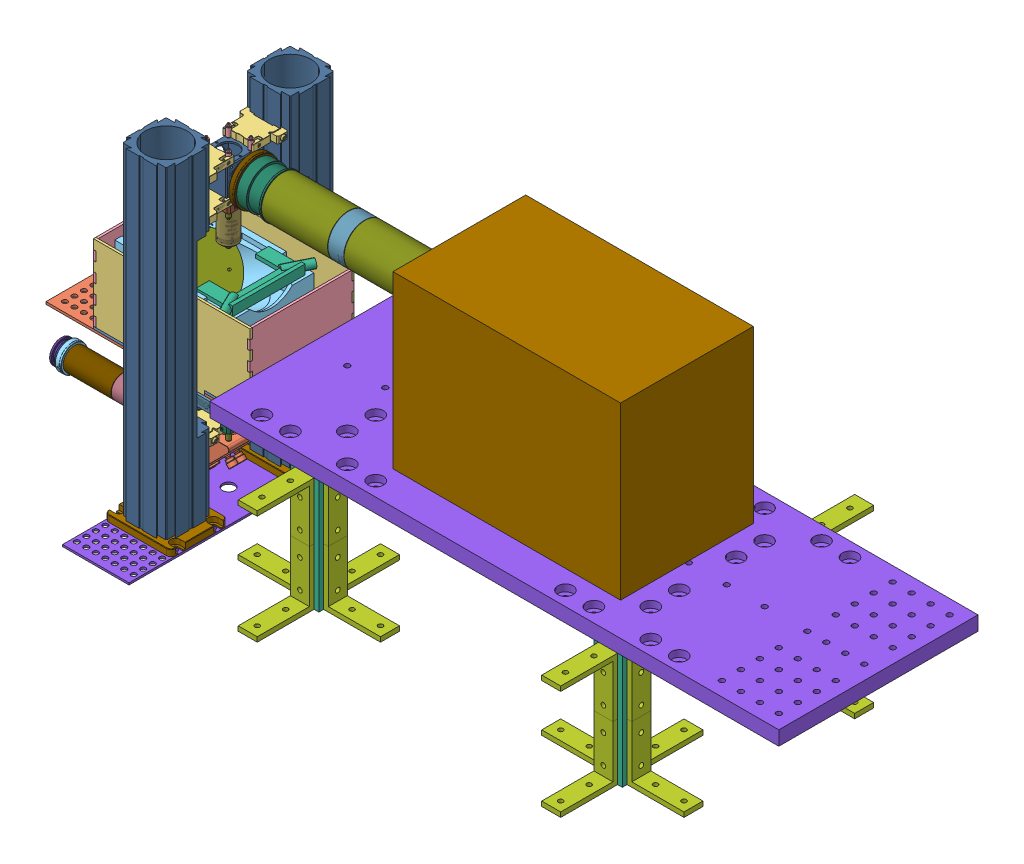
SolidWorks assembly Water Bath ABZ, configuration Default. Lengths in mm.
Overall size (1095.95 451.29 419.1).
114 component instances, 38 part files, 38 mates.
Components (placement in the parent):
- WB_0p125_BaseThreaded-1: WB_0p125_BaseThreaded [Default] at (0 3.175 0) size (209.55 3.17 139.7)
- WB_0p125_Base-1: WB_0p125_Base [Default] at origin size (273.05 3.17 139.7)
- WB_0p125_Long-1: WB_0p125_Long [Default] at (0 57.15 -69.85) size (209.55 107.95 3.17)
- WB_0p125_Long-2: WB_0p125_Long [Default] at (0 57.15 66.675) size (209.55 107.95 3.17)
- WB_0p125_Short-1: WB_0p125_Short [Default] at (101.6 57.15 0) x (0 0 1) z (0 1 0) size (139.7 3.17 107.95)
- WB_0p125_Short-2: WB_0p125_Short [Default] at (-104.775 57.15 0) x (0 0 1) z (0 1 0) size (139.7 3.17 107.95)
- 300 kHz Tank HP (5) Opticell-1: 300 kHz Tank HP (5) Opticell [Default] at (6.35 95.25 0) size (171.45 88.9 114.3)
- Opticell_Truncated-1: Opticell_Truncated [Default] at (23.9788 95.275 -0.195) size (53.01 12.75 129.72)
- HP Tx-1: HP Tx [Default] at (-41.775 64.925 0) x (0.498711 -0.863793 0.071763) z (-0.035882 0.062149 0.997422) size (83.8 58.17 83.8)
- Table SubAssembly-1: Table SubAssembly [Default] at (-31.75 -161.9485 0) x (0 0 -1) z (1 0 0) size (355.6 442.98 89.6)
  - Table-1: Table [Default] at origin size (355.6 2.54 88.9)
  - XT66P1-Solidworks-1: XT66P1-Solidworks [Default] at (-83.0224 2.286 37.592) x (-1 0 0) z (0 0 -1) size (76.2 8.89 89.28)
  - XT66P1-Solidworks-2: XT66P1-Solidworks [Default] at (83.0224 2.286 37.592) size (76.2 8.89 89.28)
  - KCB1-Solidworks-1: KCB1-Solidworks [Default] at (-24.13 99.7796 13.4747) x (0.000001 0 1) z (0 1 0) size (51.13 48.26 51.1) (hidden)
  - RCA1-Solidworks-1: RCA1-Solidworks [Default] at (-24.2926 205.6203 66.0649) x (0 0 -1) z (0 -1 0) size (56.5 73.55 8.89) (hidden)
  - RCA1-Solidworks-2: RCA1-Solidworks [Default] at (24.2926 108.2389 66.0649) x (0 0 -1) z (0 1 0) size (56.5 73.55 8.89) (hidden)
  - XT66-500-modified_v2-1: XT66-500-modified_v2 [Default] at (-83.0224 511.176 37.592) x (0 0 -1) z (0 -1 0) size (66.02 67.06 431.8)
  - XT66-500-modified_v2-2: XT66-500-modified_v2 [Default] at (83.0224 511.176 37.592) x (0 0 1) z (0 -1 0) size (66.02 67.06 431.8)
- Small Condenser Adjustable Sub-Assembly-1: Small Condenser Adjustable Sub-Assembly [Default] at (41.91 -37.4885 20.3199) x (0 -1 0) z (0 0 1) size (204.14 301.96 127)
  - LB1437-Solidworks-1: LB1437-Solidworks [Default] at (76.2 -223.413 -20.3199) x (0.879994 0 -0.474985) z (0 -1 0) size (25.4 25.4 3.05)
  - LB1761-Solidworks-1: LB1761-Solidworks [Default] at (76.2 -78.613 -20.3199) x (0.962182 0 -0.272406) z (0 -1 0) size (25.4 25.4 8.98)
  - SM1L40-Solidworks-1: SM1L40-Solidworks [Default] at (78.3398 -122.5422 -22.1696) x (-0.992854 0 -0.119336) z (0 1 0) size (30.48 30.48 105.41)
  - CSA1003-Solidworks-1: CSA1003-Solidworks [Default] at (47.6181 -122.449 -34.035) x (0 -1 0) z (0 0 1) size (71.12 13.97 71.12)
  - LCP02-Solidworks-1: LCP02-Solidworks [Default] at (20.32 -35.5599 -20.32) x (0 0 -1) z (1 0 0) size (70.75 70.61 12.7)
  - ER1-Solidworks-1: ER1-Solidworks [Default] at (36.8841 -51.9737 -4.6825) x (0 -0.925141 -0.379624) z (0 -0.379624 0.925141) size (5.99 30.48 5.99)
  - ER1-Solidworks-3: ER1-Solidworks [Default] at (36.8841 -50.6608 -33.7724) x (0 -0.769482 0.638668) z (0 0.638668 0.769482) size (5.99 30.48 5.99)
  - ER1-Solidworks-4: ER1-Solidworks [Default] at (41.8559 -21.5595 -36.5057) x (0 -0.998351 -0.057413) z (0 0.057413 -0.998351) size (5.99 30.48 5.99)
  - SM1T2-Solidworks-1: SM1T2-Solidworks [Default] at (76.2 -248.6152 -20.3199) x (0.998592 0 -0.053039) z (0 1 0) size (31.75 31.75 12.7)
  - SM1L25-Solidworks-1: SM1L25-Solidworks [Default] at (139.9124 -186.275 -15.6668) x (0 -1 0) z (-0.806632 0 -0.591053) size (67.31 30.48 30.48)
  - CP08-Solidworks-3: CP08-Solidworks [Default] at (76.2 -69.215 -20.3199) x (0 0 -1) z (0 1 0) size (41.5 40.64 8.89)
  - KCB1-Solidworks-2: KCB1-Solidworks [Default] at (100.33 -11.43 3.8101) x (-1 0 0) z (0 -1 0) size (51.13 48.26 51.1)
  - ER1-Solidworks-6: ER1-Solidworks [Default] at (36.8841 -20.7263 -3.7781) x (0 -0.795862 0.605478) z (0 0.605478 0.795862) size (5.99 30.48 5.99)
  - RCA2-Solidworks-1: RCA2-Solidworks [Default] at (68.2294 -49.0321 -29.2771) x (0 1 0) z (-1 0 0) size (56.73 41.06 8.89)
  - RCA2-Solidworks-2: RCA2-Solidworks [Default] at (68.2294 -22.0879 -11.3628) x (0 -1 0) z (-1 0 0) size (56.73 41.06 8.89)
  - ER05-Solidworks-1: ER05-Solidworks [Default] at (92.6015 -68.5259 -5.9839) x (0.310188 0 -0.950675) z (0.950675 0 0.310188) size (5.99 17.78 5.99)
  - ER05-Solidworks-2: ER05-Solidworks [Default] at (59.8613 -68.5259 -4.5371) x (-0.22668 0 0.973969) z (-0.973969 0 -0.22668) size (5.99 17.78 5.99)
  - ER05-Solidworks-3: ER05-Solidworks [Default] at (92.2659 -68.5259 -34.1935) size (5.99 17.78 5.99)
  - ER05-Solidworks-4: ER05-Solidworks [Default] at (59.7556 -68.5259 -34.7555) x (-0.375833 0 0.926687) z (-0.926687 0 -0.375833) size (5.99 17.78 5.99)
  - SM1D12D-Solidworks-1: SM1D12D-Solidworks [Default] at (81.3975 -244.783 -22.8892) x (0.973299 0 -0.22954) z (0 1 0) size (35.81 35.81 11.94)
  - SM1D12D-Solidworks-2: SM1D12D-Solidworks [Default] at (70.9424 -73.1298 -22.7639) x (-0.788375 0 -0.615195) z (0 1 0) size (35.81 35.81 11.94)
  - ER1-Solidworks-9: ER1-Solidworks [Default] at (15.1859 -4.2179 -49.5429) x (0 0.95877 -0.284182) z (0 0.284182 0.95877) size (5.99 30.48 5.99)
  - ER1-Solidworks-10: ER1-Solidworks [Default] at (15.1859 -64.6339 -49.076) x (0 0.993069 0.117534) z (0 -0.117534 0.993069) size (5.99 30.48 5.99)
  - ER1-Solidworks-11: ER1-Solidworks [Default] at (15.1859 -4.6008 10.8986) x (0 0.995869 0.090807) z (0 -0.090807 0.995869) size (5.99 30.48 5.99)
  - ER1-Solidworks-12: ER1-Solidworks [Default] at (15.1859 -64.2349 10.4858) x (0 0.96466 -0.263499) z (0 0.263499 0.96466) size (5.99 30.48 5.99)
  - OlympusCondenser-1: OlympusCondenser [Default] at (7.0104 -35.56 -20.3199) x (0 -1 0) z (0 0 -1) size (152.4 107.95 127) (hidden)
- Full Assembly Total Support-1: Full Assembly Total Support [Default] at (495.5495 41.6875 0) size (762 171.45 419.1)
  - Post SubAssembly-1: Post SubAssembly [Default] at (-254 -152.4 114.3) size (190.5 152.4 190.5)
    - Post-1: Post [Default] at origin size (38.1 152.4 38.1)
    - Hinge-1: Hinge [Default] at (-25.4 6.35 0) x (0 0 -1) z (0 -1 0) size (25.4 76.2 76.2)
    - Hinge-2: Hinge [Default] at (0 6.35 25.4) x (-1 0 0) z (0 -1 0) size (25.4 76.2 76.2)
    - Hinge-3: Hinge [Default] at (25.4 6.35 0) x (0 0 1) z (0 -1 0) size (25.4 76.2 76.2)
    - Hinge-4: Hinge [Default] at (0 6.35 -25.4) x (1 0 0) z (0 -1 0) size (25.4 76.2 76.2)
    - Hinge-5: Hinge [Default] at (25.4 146.05 0) x (0 0 1) z (-1 0 0) size (25.4 76.2 76.2)
    - Hinge-7: Hinge [Default] at (-25.4 146.05 0) x (0 0 -1) z (1 0 0) size (25.4 76.2 76.2)
    - Hinge-8: Hinge [Default] at (0 146.05 25.4) x (-1 0 0) z (0 0 -1) size (25.4 76.2 76.2)
    - Hinge-9: Hinge [Default] at (0 146.05 -25.4) size (25.4 76.2 76.2)
  - Post SubAssembly-2: Post SubAssembly [Default] at (-254 -152.4 -114.3) size (190.5 152.4 190.5)
    - Post-1: Post [Default] at origin size (38.1 152.4 38.1)
    - Hinge-1: Hinge [Default] at (-25.4 6.35 0) x (0 0 -1) z (0 -1 0) size (25.4 76.2 76.2)
    - Hinge-2: Hinge [Default] at (0 6.35 25.4) x (-1 0 0) z (0 -1 0) size (25.4 76.2 76.2)
    - Hinge-3: Hinge [Default] at (25.4 6.35 0) x (0 0 1) z (0 -1 0) size (25.4 76.2 76.2)
    - Hinge-4: Hinge [Default] at (0 6.35 -25.4) x (1 0 0) z (0 -1 0) size (25.4 76.2 76.2)
    - Hinge-5: Hinge [Default] at (25.4 146.05 0) x (0 0 1) z (-1 0 0) size (25.4 76.2 76.2)
    - Hinge-7: Hinge [Default] at (-25.4 146.05 0) x (0 0 -1) z (1 0 0) size (25.4 76.2 76.2)
    - Hinge-8: Hinge [Default] at (0 146.05 25.4) x (-1 0 0) z (0 0 -1) size (25.4 76.2 76.2)
    - Hinge-9: Hinge [Default] at (0 146.05 -25.4) size (25.4 76.2 76.2)
  - Post SubAssembly-3: Post SubAssembly [Default] at (152.4 -152.4 114.3) size (190.5 152.4 190.5)
    - Post-1: Post [Default] at origin size (38.1 152.4 38.1)
    - Hinge-1: Hinge [Default] at (-25.4 6.35 0) x (0 0 -1) z (0 -1 0) size (25.4 76.2 76.2)
    - Hinge-2: Hinge [Default] at (0 6.35 25.4) x (-1 0 0) z (0 -1 0) size (25.4 76.2 76.2)
    - Hinge-3: Hinge [Default] at (25.4 6.35 0) x (0 0 1) z (0 -1 0) size (25.4 76.2 76.2)
    - Hinge-4: Hinge [Default] at (0 6.35 -25.4) x (1 0 0) z (0 -1 0) size (25.4 76.2 76.2)
    - Hinge-5: Hinge [Default] at (25.4 146.05 0) x (0 0 1) z (-1 0 0) size (25.4 76.2 76.2)
    - Hinge-7: Hinge [Default] at (-25.4 146.05 0) x (0 0 -1) z (1 0 0) size (25.4 76.2 76.2)
    - Hinge-8: Hinge [Default] at (0 146.05 25.4) x (-1 0 0) z (0 0 -1) size (25.4 76.2 76.2)
    - Hinge-9: Hinge [Default] at (0 146.05 -25.4) size (25.4 76.2 76.2)
  - Post SubAssembly-4: Post SubAssembly [Default] at (152.4 -152.4 -114.3) size (190.5 152.4 190.5)
    - Post-1: Post [Default] at origin size (38.1 152.4 38.1)
    - Hinge-1: Hinge [Default] at (-25.4 6.35 0) x (0 0 -1) z (0 -1 0) size (25.4 76.2 76.2)
    - Hinge-2: Hinge [Default] at (0 6.35 25.4) x (-1 0 0) z (0 -1 0) size (25.4 76.2 76.2)
    - Hinge-3: Hinge [Default] at (25.4 6.35 0) x (0 0 1) z (0 -1 0) size (25.4 76.2 76.2)
    - Hinge-4: Hinge [Default] at (0 6.35 -25.4) x (1 0 0) z (0 -1 0) size (25.4 76.2 76.2)
    - Hinge-5: Hinge [Default] at (25.4 146.05 0) x (0 0 1) z (-1 0 0) size (25.4 76.2 76.2)
    - Hinge-7: Hinge [Default] at (-25.4 146.05 0) x (0 0 -1) z (1 0 0) size (25.4 76.2 76.2)
    - Hinge-8: Hinge [Default] at (0 146.05 25.4) x (-1 0 0) z (0 0 -1) size (25.4 76.2 76.2)
    - Hinge-9: Hinge [Default] at (0 146.05 -25.4) size (25.4 76.2 76.2)
  - Camera Shelf Full Support v2-1: Camera Shelf Full Support v2 [Default] at origin size (762 19.05 266.7)
- hpvx2-1: hpvx2 [Default] at (467.8011 60.7375 0.0468) size (311.15 228.6 177.8)
- Objective Sub-Assembly-1: Objective Sub-Assembly [Default] at (41.0423 -225.3982 114.3819) x (0 0 -1) z (0 -1 0) size (106.71 57.63 128.02)
  - CM1-DCH-Solidworks-1: CM1-DCH-Solidworks [Web Assembly] at (114.3818 -34.6924 -438.5894) x (0 -1 0) z (0 0 1) size (38.1 45.72 38.1)
  - CP16-Solidworks-1: CP16-Solidworks [Default] at (116.5677 -16.5858 -398.1348) x (0 -1 0) z (0 0 1) size (41.22 40.64 8.89)
  - RCA2-Solidworks-1: RCA2-Solidworks [Default] at (123.339 -21.2203 -499.1988) x (0 -1 0) z (0 0 1) size (56.73 41.06 8.89)
  - RCA2-Solidworks-2: RCA2-Solidworks [Default] at (105.4247 -48.1644 -499.1988) x (0 1 0) z (0 0 1) size (56.73 41.06 8.89)
  - N40X-NIR-Solidworks-1: N40X-NIR-Solidworks [Default] at (114.3819 -34.6923 -375.0894) x (0 0 1) z (0.875921 0.482454 0) size (61.98 27.94 27.94)
  - RCA2-Solidworks-3: RCA2-Solidworks [Default] at (105.4247 -48.1644 -452.2088) x (0 1 0) z (0 0 1) size (56.73 41.06 8.89)
  - RCA2-Solidworks-4: RCA2-Solidworks [Default] at (123.339 -21.2203 -452.2088) x (0 -1 0) z (0 0 1) size (56.73 41.06 8.89)
  - ER1-Solidworks-1: ER1-Solidworks [Default] at (100.293 -20.9473 -404.3535) x (-0.183947 -0.982936 0) z (0.982936 -0.183947 0) size (5.99 30.48 5.99)
  - ER1-Solidworks-2: ER1-Solidworks [Default] at (130.5299 -50.7349 -404.3535) x (0.020475 -0.99979 0) z (0.99979 0.020475 0) size (5.99 30.48 5.99)
  - ER1-Solidworks-3: ER1-Solidworks [Default] at (100.0093 -51.1105 -404.3535) x (-0.386185 -0.922421 0) z (0.922421 -0.386185 0) size (5.99 30.48 5.99)
  - ER1-Solidworks-4: ER1-Solidworks [Default] at (129.6817 -21.2139 -404.3535) x (-0.579753 -0.814792 0) z (0.814792 -0.579753 0) size (5.99 30.48 5.99)
  - ER05-Solidworks-1: ER05-Solidworks [Default] at (129.9725 -48.2584 -461.5035) x (0.933397 0.358845 0) z (-0.358845 0.933397 0) size (5.99 17.78 5.99)
  - ER05-Solidworks-2: ER05-Solidworks [Default] at (97.9162 -50.199 -461.5035) x (-0.886919 0.461926 0) z (-0.461926 -0.886919 0) size (5.99 17.78 5.99)
  - ER05-Solidworks-3: ER05-Solidworks [Default] at (128.9134 -21.1707 -461.5035) x (-0.900043 -0.4358 0) z (0.4358 -0.900043 0) size (5.99 17.78 5.99)
  - ER05-Solidworks-4: ER05-Solidworks [Default] at (100.2773 -18.4261 -461.5035) x (0.989892 0.141823 0) z (-0.141823 0.989892 0) size (5.99 17.78 5.99)
- Camera Sub-Assembly-1: Camera Sub-Assembly [Default] at (25.4 213.1913 0) x (0 -0.657803 -0.75319) z (-1 0 0) size (71.93 71.93 298.88)
  - SM2NFM2-Solidworks-1: SM2NFM2-Solidworks [Default] at (0 0 -285.6832) x (0 1 0) z (-1 0 0) size (63.5 16.37 63.5)
  - TTL200-S8-Solidworks-1: TTL200-S8-Solidworks [Default] at (0 0 -152.5317) size (55.88 55.88 28)
  - SM2V15-Solidworks-1: SM2V15-Solidworks [Default] at (18.0496 -29.8565 -288.422) x (0 0 -1) z (0.951776 0.306793 0) size (51.56 57.15 57.15)
  - SM2M35-Solidworks-1: SM2M35-Solidworks [Default] at (-10.7846 9.351 -219.5042) x (0.99081 -0.135264 0) z (0 0 1) size (55.88 55.88 88.9)
  - SM2M35-Solidworks-2: SM2M35-Solidworks [Default] at (-11.8362 7.9783 -108.9542) x (0.999895 -0.014459 0) z (0 0 1) size (55.88 55.88 88.9)
  - SM2V15-Solidworks-2: SM2V15-Solidworks [Default] at (-9.1968 -33.7176 -16.6413) x (0 0 1) z (-0.999373 0.035397 0) size (51.56 57.15 57.15)
  - SM1T2-Solidworks-1: SM1T2-Solidworks [Default] at (0 0 1.778) x (0.997143 -0.075539 0) z (0 0 1) size (31.75 31.75 12.7)
  - SM2A6-Solidworks-2: SM2A6-Solidworks [Default] at (0 0 -9.144) size (51.69 51.69 5.08)
  - SM2D25D-Solidworks-1: SM2D25D-Solidworks [Default] at (-6.3593 1.1475 -12.9462) x (-1 0 0) z (0 0 -1) size (60.96 60.96 12.32)
Mates (geometry in assembly coordinates):
- Coincident1: coincident aligned: plane of WB_0p125_BaseThreaded-1 through (-101.6 6.35 66.675) normal (0 0 1); plane of WB_0p125_Base-1 through (-101.6 3.175 66.675) normal (0 0 1)
- Coincident2: coincident aligned: plane of WB_0p125_BaseThreaded-1 through (101.6 6.35 66.675) normal (1 0 0); plane of WB_0p125_Base-1 through (101.6 3.175 66.675) normal (1 0 0)
- Coincident3: coincident anti-aligned: plane of WB_0p125_BaseThreaded-1 through (0 3.175 0) normal (0 -1 0); plane of WB_0p125_Base-1 through (0 3.175 0) normal (0 1 0)
- Coincident4: coordinate: point of WB_0p125_Base-1; point of assembly
- Coincident5: coincident aligned: plane of WB_0p125_BaseThreaded-1 through (101.6 6.35 66.675) normal (1 0 0); plane of WB_0p125_Long-2 through (101.6 6.35 69.85) normal (1 0 0)
- Coincident6: coincident anti-aligned: plane of WB_0p125_BaseThreaded-1 through (0 6.35 0) normal (0 1 0); plane of WB_0p125_Long-2 through (-101.6 6.35 69.85) normal (0 -1 0)
- Coincident8: coincident anti-aligned: plane of WB_0p125_BaseThreaded-1 through (0 6.35 0) normal (0 1 0); plane of WB_0p125_Long-1 through (-101.6 6.35 -66.675) normal (0 -1 0)
- Coincident9: coincident aligned: plane of WB_0p125_BaseThreaded-1 through (-101.6 6.35 66.675) normal (-1 0 0); plane of WB_0p125_Long-1 through (-101.6 6.35 -66.675) normal (-1 0 0)
- Coincident11: coincident anti-aligned: plane of WB_0p125_BaseThreaded-1 through (-101.6 6.35 66.675) normal (-1 0 0); plane of WB_0p125_Short-2 through (-101.6 57.15 0) normal (1 0 0)
- Coincident12: coincident anti-aligned: plane of WB_0p125_BaseThreaded-1 through (0 6.35 0) normal (0 1 0); plane of WB_0p125_Short-2 through (-101.6 6.35 -66.675) normal (0 -1 0)
- Coincident14: coincident anti-aligned: plane of WB_0p125_Long-2 through (0 57.15 66.675) normal (0 0 -1); plane of WB_0p125_Short-2 through (-101.6 107.95 66.675) normal (0 0 1)
- Coincident16: coincident anti-aligned: plane of WB_0p125_Long-2 through (0 57.15 66.675) normal (0 0 -1); plane of WB_0p125_Short-1 through (104.775 107.95 66.675) normal (0 0 1)
- Coincident18: coincident anti-aligned: plane of WB_0p125_Long-1 through (0 57.15 -66.675) normal (0 0 1); plane of WB_0p125_Short-2 through (-101.6 107.95 -66.675) normal (0 0 -1)
- Coincident19: coincident anti-aligned: plane of WB_0p125_BaseThreaded-1 through (-101.6 6.35 -66.675) normal (0 0 -1); plane of WB_0p125_Long-1 through (0 57.15 -66.675) normal (0 0 1)
- Coincident20: coincident aligned: plane of WB_0p125_Long-2 through (104.775 107.95 66.675) normal (1 0 0); plane of WB_0p125_Short-1 through (104.775 57.15 0) normal (1 0 0)
- Coincident21: coincident aligned: plane of WB_0p125_Base-1 through (0 0 0) normal (0 -1 0); plane of WB_0p125_Short-1 through (104.775 0 9.525) normal (0 -1 0)
- Concentric3: concentric aligned: circle of WB_0p125_BaseThreaded-1; circle of 300 kHz Tank HP (5) Opticell-1
- Concentric4: concentric aligned: circle of WB_0p125_BaseThreaded-1; circle of 300 kHz Tank HP (5) Opticell-1
- Coincident23: coincident anti-aligned: plane of WB_0p125_BaseThreaded-1 through (0 6.35 0) normal (0 1 0); plane of 300 kHz Tank HP (5) Opticell-1 through (6.35 6.35 0) normal (0 -1 0)
- Coincident24: coincident anti-aligned: plane of 300 kHz Tank HP (5) Opticell-1 through (6.35 88.9 0) normal (0 1 0); plane of Opticell_Truncated-1 through (23.9788 88.9 -0.195) normal (0 -1 0)
- Coincident25: coincident: plane of 300 kHz Tank HP (5) Opticell-1 through (-12.0762 88.9 -48.895) normal (1 0 0); plane of Opticell_Truncated-1 through (-12.0762 97.775 48.505) normal (-1 0 0)
- Coincident26: coincident anti-aligned: plane of 300 kHz Tank HP (5) Opticell-1 through (-24.7762 88.9 -48.895) normal (0 0 1); plane of Opticell_Truncated-1 through (-12.0762 97.775 -48.895) normal (0 0 -1)
- Concentric5: concentric aligned: cylinder of 300 kHz Tank HP (5) Opticell-1 through (-41.775 64.925 0) axis (-0.866025 -0.5 0) radius 42.545; cylinder of HP Tx-1 through (-41.775 64.925 0) axis (-0.866025 -0.5 0) radius 41.9
- Coincident27: coincident anti-aligned: plane of 300 kHz Tank HP (5) Opticell-1 through (-43.7925 68.4194 0) normal (0.866025 0.5 0); plane of HP Tx-1 through (-41.775 64.925 0) normal (-0.866025 -0.5 0)
- Coincident28: coincident anti-aligned: plane of Table SubAssembly-1/Table-1 through (-31.75 -161.9485 0) normal (0 0 -1); plane of assembly through (0 0 0) normal (0 0 1)
- Concentric6: concentric aligned: circle of 300 kHz Tank HP (5) Opticell-1; circle of Table SubAssembly-1/Table-1
- Concentric7: concentric aligned: circle of Table SubAssembly-1/Table-1; circle of Small Condenser Adjustable Sub-Assembly-1/OlympusCondenser-1
- Parallel1: parallel aligned: plane of Table SubAssembly-1/XT66-500-modified_v2-1 through (-14.496 -150.7725 116.5515) normal (0 0 1); plane of Small Condenser Adjustable Sub-Assembly-1/CSA1003-Solidworks-1 through (41.91 -37.4885 35.56) normal (0 0 1)
- Distance1: distance = 25.4 mm anti-aligned: plane of Small Condenser Adjustable Sub-Assembly-1/CP08-Solidworks-3 through (-22.86 -134.0085 18.034) normal (0 -1 0); plane of Table SubAssembly-1/Table-1 through (-31.75 -159.4085 0) normal (0 1 0)
- Concentric8: concentric aligned: circle of Table SubAssembly-1/Table-1; circle of Objective Sub-Assembly-1/N40X-NIR-Solidworks-1
- Parallel2: parallel aligned: plane of Table SubAssembly-1/XT66-500-modified_v2-1 through (-27.1658 -150.7725 103.3604) normal (-1 0 0); plane of Objective Sub-Assembly-1/CM1-DCH-Solidworks-1 through (-12.7 194.1413 -19.05) normal (-1 0 0)
- Concentric9: concentric aligned: cylinder of Objective Sub-Assembly-1/CM1-DCH-Solidworks-1 through (-12.7 213.1913 0) axis (-1 0 0) radius 12.8524; cylinder of Camera Sub-Assembly-1/SM2M35-Solidworks-2 through (125.1967 213.1913 0) axis (-1 0 0) radius 27.94
- Coincident29: coincident anti-aligned: plane of Objective Sub-Assembly-1/CM1-DCH-Solidworks-1 through (25.4 194.1413 -19.05) normal (1 0 0); plane of Camera Sub-Assembly-1/SM1T2-Solidworks-1 through (25.4 205.0538 -10.8774) normal (-1 0 0)
- Concentric10: concentric aligned: cylinder of hpvx2-1 through (315.4011 213.1375 0.0468) axis (1 0 0) radius 29.1375; cylinder of Camera Sub-Assembly-1/SM2V15-Solidworks-1 through (310.9561 213.1375 0.0468) axis (1 0 0) radius 27.94
- Coincident30: coincident anti-aligned: plane of hpvx2-1 through (315.4011 289.3375 88.9468) normal (-1 0 0); plane of Camera Sub-Assembly-1/SM2NFM2-Solidworks-1 through (315.4011 213.1913 0) normal (1 0 0)
- Parallel3: parallel aligned: plane of Table SubAssembly-1/XT66-500-modified_v2-2 through (-27.1658 281.0275 -49.4934) normal (0 1 0); plane of hpvx2-1 through (467.8011 289.3375 0.0468) normal (0 1 0)
- Coincident31: coincident anti-aligned: plane of Full Assembly Total Support-1/Camera Shelf Full Support v2-1 through (495.5495 60.7375 0) normal (0 1 0); plane of hpvx2-1 through (467.8011 60.7375 0.0468) normal (0 -1 0)
- Coincident32: coincident aligned: plane of Full Assembly Total Support-1/Camera Shelf Full Support v2-1 through (495.5495 41.6875 0) normal (0 0 1); plane of assembly through (0 0 0) normal (0 0 1)
